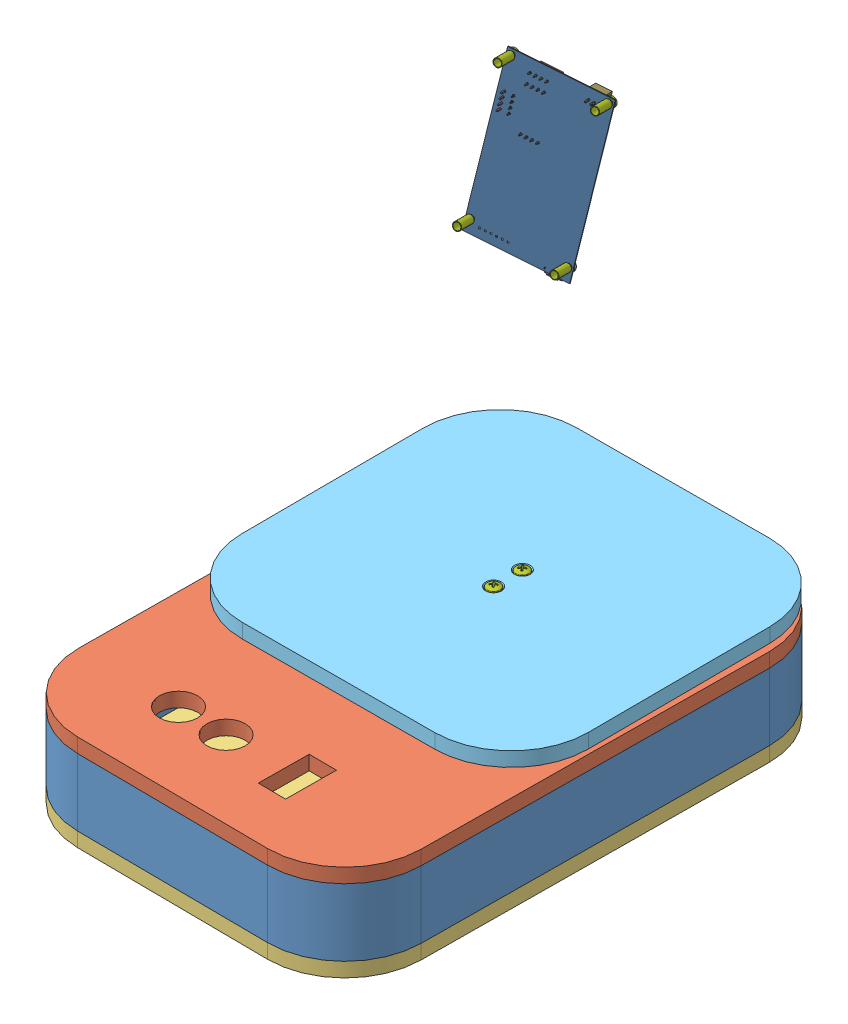
SolidWorks assembly Mainv1, configuration Default. Lengths in mm.
Overall size (261.27 140.54 358.53).
175 component instances, 43 part files, 26 mates.
Components (placement in the parent):
- mail wall-1: mail wall [Default] at (468.1099 74.0645 -181.95) x (-0.999962 0 -0.008727) z (0.008727 0 -0.999962) size (180 35 260)
- top lid-1: top lid [Default] at (468.1099 116.5645 -181.95) x (-0.999962 0 -0.008727) z (0.008727 0 -0.999962) size (180 7.5 260)
- bottom lid-2: bottom lid [Default] at (468.1099 31.5645 -181.95) x (0.999962 0 0.008727) z (-0.008727 0 0.999962) size (180 7.5 260)
- Loadcell-1kg-No Name.step-1: Loadcell-1kg-No Name.step [Default] at (468.4825 94.8439 -197.5959) x (0 0 1) z (-1 0 0) size (91.8 14.23 13.91)
- tray-1: tray [Default] at (468.6751 134.9439 -266.3463) x (0.999991 0 -0.00428) z (0.00428 0 0.999991) size (180 7.5 175)
- Part5-1: Part5 [Default] at origin size (12.6 12.5 27.5)
- pan cross head_am-1: pan cross head_am [B18.6.7M - M3.5 x 0.6 x 35 Type I Cross Recessed PHMS --35N] at (468.4825 128.4614 -232.8459) x (0 -1 0) z (-0.788636 0 0.61486) size (37.57 7 7)
- pan cross head_am-3: pan cross head_am [B18.6.7M - M3.5 x 0.6 x 35 Type I Cross Recessed PHMS --35N] at (468.4825 128.5554 -217.8459) x (0 -1 0) z (0.792721 0 -0.609585) size (37.57 7 7)
- Part1-1: Part1 [Default] at origin size (50 22.7 32.99)
- hex bolt_am-1: hex bolt_am [B18.2.3.5M - Hex bolt M5 x 0.8 x 35 --16N] at (468.8184 72.2139 -162.6607) x (0 1 0) z (0 0 1) size (38.58 9.24 8)
- hex bolt_am-2: hex bolt_am [B18.2.3.5M - Hex bolt M5 x 0.8 x 35 --16N] at (468.8184 72.2139 -177.7301) x (0 1 0) z (0 0 1) size (38.58 9.24 8)
- pcb.step-1: pcb.step [Default] at (347.6655 123.4151 -378.6091) x (-0.974446 0.114203 0.193422) z (-0.214397 -0.216049 -0.952553) size (48.01 79.98 16.61)
  - Board.step-1: Board.step [Default] at origin size (48.01 78.74 0.41)
    - Open CASCADE STEP translator 7.5 2.1.1.step-1: Open CASCADE STEP translator 7.5 2.1.1.step [Default] at (0 0 -0.4115) size (48.01 78.74 0.41)
  - HX711 out.step-1: HX711 out.step [Default] at origin size (10.16 2.54 10.59)
    - Header_4.step-1: Header_4.step [Default] at (27.685 46.598 -0.0051) x (0 -1 0) z (-1 0 0) size (2.54 10.59 10.16)
      - header.step-1: header.step [Default] at origin size (2.54 10.59 2.54)
        - header-0.step-1: header-0.step [Default] at origin size (2.54 8.5 2.54)
        - pin.step-1: pin.step [Default] at (-1.4 0 0) size (0.4 10 1.99)
      - header.step-2: header.step [Default] at (0 0 -2.54) size (2.54 10.59 2.54)
        - header-0.step-1: header-0.step [Default] at origin size (2.54 8.5 2.54)
        - pin.step-1: pin.step [Default] at (-1.4 0 0) size (0.4 10 1.99)
      - header.step-3: header.step [Default] at (0 0 -5.08) size (2.54 10.59 2.54)
        - header-0.step-1: header-0.step [Default] at origin size (2.54 8.5 2.54)
        - pin.step-1: pin.step [Default] at (-1.4 0 0) size (0.4 10 1.99)
      - header.step-4: header.step [Default] at (0 0 -7.62) size (2.54 10.59 2.54)
        - header-0.step-1: header-0.step [Default] at origin size (2.54 8.5 2.54)
        - pin.step-1: pin.step [Default] at (-1.4 0 0) size (0.4 10 1.99)
  - HX711_lc.step-1: HX711_lc.step [Default] at origin size (10.16 2.54 10.59)
    - Header_4.step-1: Header_4.step [Default] at (30.23 66.915 -0.0051) x (0 -1 0) z (-1 0 0) size (2.54 10.59 10.16)
      - header.step-1: header.step [Default] at origin size (2.54 10.59 2.54)
        - header-0.step-1: header-0.step [Default] at origin size (2.54 8.5 2.54)
        - pin.step-1: pin.step [Default] at (-1.4 0 0) size (0.4 10 1.99)
      - header.step-2: header.step [Default] at (0 0 -2.54) size (2.54 10.59 2.54)
        - header-0.step-1: header-0.step [Default] at origin size (2.54 8.5 2.54)
        - pin.step-1: pin.step [Default] at (-1.4 0 0) size (0.4 10 1.99)
      - header.step-3: header.step [Default] at (0 0 -5.08) size (2.54 10.59 2.54)
        - header-0.step-1: header-0.step [Default] at origin size (2.54 8.5 2.54)
        - pin.step-1: pin.step [Default] at (-1.4 0 0) size (0.4 10 1.99)
      - header.step-4: header.step [Default] at (0 0 -7.62) size (2.54 10.59 2.54)
        - header-0.step-1: header-0.step [Default] at origin size (2.54 8.5 2.54)
        - pin.step-1: pin.step [Default] at (-1.4 0 0) size (0.4 10 1.99)
  - usb 2.0.step-1: usb 2.0.step [Default] at origin size (7.8 5.5 3.71)
    - USB3090-30-A--3DModel-STEP-56544.step-1: USB3090-30-A--3DModel-STEP-56544.step [Default] at (7.762 1.514 0) x (1 0 0) z (0 -1 0) size (7.8 3.71 5.5)
  - R 470.step-1: R 470.step [Default] at origin size (2 1.25 0.6)
    - 6201218720.step-1: 6201218720.step [Default] at (15.687 7.62 0) x (1 0 0) z (0 0 1) size (2 1.25 0.6)
      - term1.step-1: term1.step [Default] at (-1 -0.625 0) size (0.35 1.25 0.6)
      - term2.step-1: term2.step [Default] at (0.65 -0.625 0) size (0.35 1.25 0.6)
      - body.step-1: body.step [Default] at (-0.65 -0.6125 0.006) size (1.3 1.22 0.59)
  - R 47k.step-1: R 47k.step [Default] at origin size (2 1.25 0.6)
    - 6062674512.step-1: 6062674512.step [Default] at (18.862 49.53 0) x (-1 0 0) z (0 0 1) size (2 1.25 0.6)
      - term1-1.step-1: term1-1.step [Default] at (-1 -0.625 0) size (0.35 1.25 0.6)
      - term2-2.step-1: term2-2.step [Default] at (0.65 -0.625 0) size (0.35 1.25 0.6)
      - body-3.step-1: body-3.step [Default] at (-0.65 -0.6125 0.006) size (1.3 1.22 0.59)
  - R 15k.step-1: R 15k.step [Default] at origin size (2 1.25 0.6)
    - 7267289360.step-1: 7267289360.step [Default] at (18.937 59.563 0) x (-1 0 0) z (0 0 1) size (2 1.25 0.6)
      - solidBody.step-1: solidBody.step [Default] at origin size (1.95 1.25 0.55)
      - Terminal.step-1: Terminal.step [Default] at origin size (2 1.25 0.6)
      - solidTop.step-1: solidTop.step [Default] at origin size (1.2 1.25 0.02)
  - R5-10K.step-1: R5-10K.step [Default] at origin size (1.6 0.8 0.55)
    - CRG0603F10K_10.step-1: CRG0603F10K_10.step [Default] at (45.212 17.526 0) x (1 0 0) z (0 -1 0) size (1.6 0.55 0.8)
  - R4-10K.step-1: R4-10K.step [Default] at origin size (1.6 0.8 0.55)
    - CRG0603F10K_10.step-1: CRG0603F10K_10.step [Default] at (45.212 22.7965 0) x (-1 0 0) z (0 1 0) size (1.6 0.55 0.8)
  - R3-10K.step-1: R3-10K.step [Default] at origin size (1.6 0.8 0.55)
    - CRG0603F10K_10.step-1: CRG0603F10K_10.step [Default] at (45.212 28.067 0) x (1 0 0) z (0 -1 0) size (1.6 0.55 0.8)
  - R 2k.step-1: R 2k.step [Default] at origin size (2 1.25 0.6)
    - 6062674512.step-1: 6062674512.step [Default] at (15.814 12.319 0) x (-1 0 0) z (0 0 1) size (2 1.25 0.6)
      - term1-1.step-1: term1-1.step [Default] at (-1 -0.625 0) size (0.35 1.25 0.6)
      - term2-2.step-1: term2-2.step [Default] at (0.65 -0.625 0) size (0.35 1.25 0.6)
      - body-3.step-1: body-3.step [Default] at (-0.65 -0.6125 0.006) size (1.3 1.22 0.59)
  - R2-10K.step-1: R2-10K.step [Default] at origin size (1.6 0.8 0.55)
    - CRG0603F10K_10.step-1: CRG0603F10K_10.step [Default] at (22.733 36.195 0) x (-1 0 0) z (0 1 0) size (1.6 0.55 0.8)
  - R1-10K.step-1: R1-10K.step [Default] at origin size (1.6 0.8 0.55)
    - CRG0603F10K_10.step-1: CRG0603F10K_10.step [Default] at (22.733 42.545 0) x (-1 0 0) z (0 1 0) size (1.6 0.55 0.8)
  - MCP73831.step-1: MCP73831.step [Default] at origin size (2.7 2.9 1.45)
    - MCP73831T-5ACI_OT.step-1: MCP73831T-5ACI_OT.step [Default] at (8.255 12.012 0) x (0 -1 0) z (-1 0 0) size (2.9 1.45 2.7)
  - LED.step-1: LED.step [Default] at origin size (3 1 2)
    - KPA-3010CGCK-Base.step-1: KPA-3010CGCK-Base.step [Default] at (16.51 1.651 0.508) x (-1 0 0) z (0 0 -1) size (2.16 1 1.02)
    - KPA-3010CGCK-Base-4.step-1: KPA-3010CGCK-Base-4.step [Default] at (16.51 1.651 0.508) x (-1 0 0) z (0 0 -1) size (3 1 1.22)
    - KPA-3010CGCK-Base-5.step-1: KPA-3010CGCK-Base-5.step [Default] at (16.51 1.651 0.508) x (-1 0 0) z (0 0 -1) size (0.9 1 0)
    - KPA-3010CGCK-Base-6.step-1: KPA-3010CGCK-Base-6.step [Default] at (16.51 1.651 0.508) x (-1 0 0) z (0 0 -1) size (0.8 1 0.02)
    - KPA-3010CGCK-Base-7.step-1: KPA-3010CGCK-Base-7.step [Default] at (16.51 1.651 0.508) x (-1 0 0) z (0 0 -1) size (2.96 1 0.96)
  - battery.step-1: battery.step [Default] at origin size (7.4 5.75 10.4)
    - 6062675712.step-1: 6062675712.step [Default] at (9.274 74.295 0) x (1 0 0) z (0 -1 0) size (7.4 10.4 5.75)
  - load cell.step-1: load cell.step [Default] at origin size (10.16 2.54 10.59)
    - Header_4.step-1: Header_4.step [Default] at (30.099 71.755 -0.0051) x (0 -1 0) z (-1 0 0) size (2.54 10.59 10.16)
      - header.step-1: header.step [Default] at origin size (2.54 10.59 2.54)
        - header-0.step-1: header-0.step [Default] at origin size (2.54 8.5 2.54)
        - pin.step-1: pin.step [Default] at (-1.4 0 0) size (0.4 10 1.99)
      - header.step-2: header.step [Default] at (0 0 -2.54) size (2.54 10.59 2.54)
        - header-0.step-1: header-0.step [Default] at origin size (2.54 8.5 2.54)
        - pin.step-1: pin.step [Default] at (-1.4 0 0) size (0.4 10 1.99)
      - header.step-3: header.step [Default] at (0 0 -5.08) size (2.54 10.59 2.54)
        - header-0.step-1: header-0.step [Default] at origin size (2.54 8.5 2.54)
        - pin.step-1: pin.step [Default] at (-1.4 0 0) size (0.4 10 1.99)
      - header.step-4: header.step [Default] at (0 0 -7.62) size (2.54 10.59 2.54)
        - header-0.step-1: header-0.step [Default] at origin size (2.54 8.5 2.54)
        - pin.step-1: pin.step [Default] at (-1.4 0 0) size (0.4 10 1.99)
  - buttons.step-1: buttons.step [Default] at origin size (2.54 10.16 10.59)
    - Header_4.step-1: Header_4.step [Default] at (39.497 59.817 -0.0051) x (-1 0 0) z (0 1 0) size (2.54 10.59 10.16)
      - header.step-1: header.step [Default] at origin size (2.54 10.59 2.54)
        - header-0.step-1: header-0.step [Default] at origin size (2.54 8.5 2.54)
        - pin.step-1: pin.step [Default] at (-1.4 0 0) size (0.4 10 1.99)
      - header.step-2: header.step [Default] at (0 0 -2.54) size (2.54 10.59 2.54)
        - header-0.step-1: header-0.step [Default] at origin size (2.54 8.5 2.54)
        - pin.step-1: pin.step [Default] at (-1.4 0 0) size (0.4 10 1.99)
      - header.step-3: header.step [Default] at (0 0 -5.08) size (2.54 10.59 2.54)
        - header-0.step-1: header-0.step [Default] at origin size (2.54 8.5 2.54)
        - pin.step-1: pin.step [Default] at (-1.4 0 0) size (0.4 10 1.99)
      - header.step-4: header.step [Default] at (0 0 -7.62) size (2.54 10.59 2.54)
        - header-0.step-1: header-0.step [Default] at origin size (2.54 8.5 2.54)
        - pin.step-1: pin.step [Default] at (-1.4 0 0) size (0.4 10 1.99)
  - OLED.step-1: OLED.step [Default] at origin size (2.54 10.16 16)
    - MTSW-104-22-S-S-420.step-1: MTSW-104-22-S-S-420.step [Default] at (44.831 57.277 0) x (0 -1 0) z (-1 0 0) size (10.16 16 2.54)
      - MTSW-104-22-S-420.step-1: MTSW-104-22-S-420.step [Default] at (0 -2.794 0) size (8.51 16 0.89)
      - MTSW-104-22-S-S-420_body.step-1: MTSW-104-22-S-S-420_body.step [Default] at origin size (10.16 2.54 2.54)
  - ESP-12F.step-1: ESP-12F.step [Default] at origin size (17.7 24.9 3.1)
    - ESP-12F-8.step-1: ESP-12F-8.step [Default] at (33.909 28.956 0) x (1 0 0) z (0 -1 0) size (17.7 3.1 24.9)
  - C5-4.7uF.step-1: C5-4.7uF.step [Default] at origin size (2 1.25 1.45)
    - 885012107013.step-1: 885012107013.step [Default] at (10.345 18.923 0) x (-1 0 0) z (0 0 1) size (2 1.25 1.45)
      - Fillet1.step-1: Fillet1.step [Default] at origin size (0.5 1.25 1.45)
      - Fillet2.step-1: Fillet2.step [Default] at origin size (0.5 1.25 1.45)
      - body2.step-1: body2.step [Default] at origin size (1 1.22 1.42)
  - C4-4.7uF.step-1: C4-4.7uF.step [Default] at origin size (2 1.25 1.45)
    - 885012107013.step-1: 885012107013.step [Default] at (11.245 26.543 0) x (1 0 0) z (0 0 1) size (2 1.25 1.45)
      - Fillet1.step-1: Fillet1.step [Default] at origin size (0.5 1.25 1.45)
      - Fillet2.step-1: Fillet2.step [Default] at origin size (0.5 1.25 1.45)
      - body2.step-1: body2.step [Default] at origin size (1 1.22 1.42)
  - C3-10uF.step-1: C3-10uF.step [Default] at origin size (5.3 4.5 5.5)
    - 865080340001.step-1: 865080340001.step [Default] at (10.737 64.643 0) x (-1 0 0) z (0 0 1) size (5.3 4.5 5.5)
      - Base.step-1: Base.step [Default] at origin size (4.5 4.5 1.6)
      - Pin1Fillet.step-1: Pin1Fillet.step [Default] at origin size (2.25 0.75 0.3)
      - Pin2Fillet.step-1: Pin2Fillet.step [Default] at origin size (2.25 0.75 0.3)
      - Fillet.step-1: Fillet.step [Default] at origin size (4.2 4.2 4.4)
    - 865080340001.step-2: 865080340001.step [Default] at (10.737 64.643 0) x (-1 0 0) z (0 0 1) size (5.3 4.5 5.5)
      - Base.step-1: Base.step [Default] at origin size (4.5 4.5 1.6)
      - Pin1Fillet.step-1: Pin1Fillet.step [Default] at origin size (2.25 0.75 0.3)
      - Pin2Fillet.step-1: Pin2Fillet.step [Default] at origin size (2.25 0.75 0.3)
      - Fillet.step-1: Fillet.step [Default] at origin size (4.2 4.2 4.4)
  - C2-10uF.step-1: C2-10uF.step [Default] at origin size (5.3 4.5 5.5)
    - 865080340001.step-1: 865080340001.step [Default] at (10.737 44.069 0) x (-1 0 0) z (0 0 1) size (5.3 4.5 5.5)
      - Base.step-1: Base.step [Default] at origin size (4.5 4.5 1.6)
      - Pin1Fillet.step-1: Pin1Fillet.step [Default] at origin size (2.25 0.75 0.3)
      - Pin2Fillet.step-1: Pin2Fillet.step [Default] at origin size (2.25 0.75 0.3)
      - Fillet.step-1: Fillet.step [Default] at origin size (4.2 4.2 4.4)
    - 865080340001.step-2: 865080340001.step [Default] at (10.737 44.069 0) x (-1 0 0) z (0 0 1) size (5.3 4.5 5.5)
      - Base.step-1: Base.step [Default] at origin size (4.5 4.5 1.6)
      - Pin1Fillet.step-1: Pin1Fillet.step [Default] at origin size (2.25 0.75 0.3)
      - Pin2Fillet.step-1: Pin2Fillet.step [Default] at origin size (2.25 0.75 0.3)
      - Fillet.step-1: Fillet.step [Default] at origin size (4.2 4.2 4.4)
  - C1-10uF.step-1: C1-10uF.step [Default] at origin size (5.3 4.5 5.5)
    - 865080340001.step-1: 865080340001.step [Default] at (33.583 11.303 0) x (-1 0 0) z (0 0 1) size (5.3 4.5 5.5)
      - Base.step-1: Base.step [Default] at origin size (4.5 4.5 1.6)
      - Pin1Fillet.step-1: Pin1Fillet.step [Default] at origin size (2.25 0.75 0.3)
      - Pin2Fillet.step-1: Pin2Fillet.step [Default] at origin size (2.25 0.75 0.3)
      - Fillet.step-1: Fillet.step [Default] at origin size (4.2 4.2 4.4)
    - 865080340001.step-2: 865080340001.step [Default] at (33.583 11.303 0) x (-1 0 0) z (0 0 1) size (5.3 4.5 5.5)
      - Base.step-1: Base.step [Default] at origin size (4.5 4.5 1.6)
      - Pin1Fillet.step-1: Pin1Fillet.step [Default] at origin size (2.25 0.75 0.3)
      - Pin2Fillet.step-1: Pin2Fillet.step [Default] at origin size (2.25 0.75 0.3)
      - Fillet.step-1: Fillet.step [Default] at origin size (4.2 4.2 4.4)
  - TC2117.step-1: TC2117.step [Default] at origin size (7.13 5.32 1.17)
    - TC2117-3.3VDBTR.step-1: TC2117-3.3VDBTR.step [Default] at (10.864 54.356 0) x (-1 0 0) z (0 0 1) size (7 5.32 1.17)
      - body.step-1: body.step [Default] at origin size (1.3 1.22 0.59)
      - PinsArrayL.step-1: PinsArrayL.step [Default] at origin size (1.75 5.32 1.17)
      - FilletPinR.step-1: FilletPinR.step [Default] at origin size (1.75 3 1.17)
    - TC2117-3.3VDBTR.step-2: TC2117-3.3VDBTR.step [Default] at (10.737 54.356 0) x (-1 0 0) z (0 0 1) size (7 5.32 1.17)
      - body.step-1: body.step [Default] at origin size (1.3 1.22 0.59)
      - PinsArrayL.step-1: PinsArrayL.step [Default] at origin size (1.75 5.32 1.17)
      - FilletPinR.step-1: FilletPinR.step [Default] at origin size (1.75 3 1.17)
- Part36-1: Part36 [Default] at origin size (53.08 79 35.65)
- pan cross head_am-4: pan cross head_am [B18.6.7M - M2.5 x 0.45 x 5 Type I Cross Recessed PHMS --5N] at (303.2042 134.2026 -373.2533) x (0.214397 0.216049 0.952553) z (-0.952107 -0.171442 0.253181) size (7.07 5 5)
- pan cross head_am-5: pan cross head_am [B18.6.7M - M2.5 x 0.45 x 5 Type I Cross Recessed PHMS --5N] at (307.9009 202.1811 -389.7286) x (0.214397 0.216049 0.952553) z (-0.586235 0.808507 -0.05143) size (7.07 5 5)
- pan cross head_am-6: pan cross head_am [B18.6.7M - M2.5 x 0.45 x 5 Type I Cross Recessed PHMS --5N] at (350.2335 197.3439 -398.1596) x (0.214397 0.216049 0.952553) z (0.724601 0.618774 -0.303435) size (7.07 5 5)
- pan cross head_am-7: pan cross head_am [B18.6.7M - M2.5 x 0.45 x 5 Type I Cross Recessed PHMS --5N] at (345.5283 129.2423 -381.6544) x (0.214397 0.216049 0.952553) z (-0.921974 0.36675 0.124331) size (7.07 5 5)
Mates (geometry in assembly coordinates):
- Coincident5: coincident anti-aligned: plane of Loadcell-1kg-No Name.step-1 through (468.4825 107.4439 -197.5959) normal (0 1 0); plane of Part5-1 through (0 107.4439 0) normal (0 -1 0)
- Coincident6: coincident anti-aligned: line of Loadcell-1kg-No Name.step-1 through (474.7825 107.4439 -237.5959) axis (-1 0 0); line of Part5-1 through (462.1825 107.4439 -237.5959) axis (1 0 0)
- Coincident8: coincident aligned: line of Loadcell-1kg-No Name.step-1 through (474.7825 107.4439 -157.5959) axis (0 0 -1); line of Part5-1 through (474.7825 107.4439 -210.0959) axis (0 0 -1)
- Concentric12: concentric aligned: cylinder of Part5-1 through (468.4825 127.4439 -232.8459) axis (0 1 0) radius 1.85; cylinder of pan cross head_am-1 through (468.4825 153.8614 -232.8459) axis (0 1 0) radius 1.75
- Coincident9: coincident aligned: cylinder of tray-1 through (468.4825 127.4439 -232.8459) axis (0 1 0) radius 1.85; circle of Part5-1
- Concentric15: concentric aligned: circle of tray-1; cylinder of pan cross head_am-3 through (468.4825 153.9554 -217.8459) axis (0 1 0) radius 1.75
- Concentric17: concentric aligned: cylinder of Part1-1 through (468.8184 72.1439 -162.6607) axis (0 -1 0) radius 2.65; cylinder of hex bolt_am-1 through (468.8184 72.2139 -162.6607) axis (0 -1 0) radius 2.5
- Concentric18: concentric aligned: cylinder of Part1-1 through (468.8184 72.1439 -177.7301) axis (0 -1 0) radius 2.65; cylinder of hex bolt_am-2 through (468.8184 72.2139 -177.7301) axis (0 -1 0) radius 2.5
- Coincident10: coincident anti-aligned: plane of Part1-1 through (471.4684 75.7939 -177.7301) normal (0 -1 0); plane of hex bolt_am-2 through (464.1996 75.7939 -177.7301) normal (0 1 0)
- Coincident11: coincident anti-aligned: plane of Part1-1 through (471.4684 75.7939 -162.6607) normal (0 -1 0); plane of hex bolt_am-1 through (464.1996 75.7939 -162.6607) normal (0 1 0)
- Coincident16: coincident anti-aligned: line of mail wall-1 through (557.3211 109.0645 -91.168) axis (0.008727 0 -0.999962); line of top lid-1 through (558.8919 109.0645 -271.1612) axis (-0.008727 0 0.999962)
- Coincident17: coincident aligned: line of mail wall-1 through (516.9736 109.0645 -51.5186) axis (-0.999962 0 -0.008727); line of top lid-1 through (516.9736 109.0645 -51.5186) axis (-0.999962 0 -0.008727)
- Coincident18: coincident anti-aligned: line of mail wall-1 through (516.9736 74.0645 -51.5186) axis (-0.999962 0 -0.008727); line of bottom lid-2 through (416.9774 74.0645 -52.3913) axis (0.999962 0 0.008727)
- Coincident19: coincident aligned: line of mail wall-1 through (557.3211 74.0645 -91.168) axis (0.008727 0 -0.999962); line of bottom lid-2 through (557.3211 74.0645 -91.168) axis (0.008727 0 -0.999962)
- Concentric19: concentric aligned: circle of pcb.step-1/Board.step-1/Open CASCADE STEP translator 7.5 2.1.1.step-1; cylinder of Part36-1 through (352.9159 200.047 -386.2417) axis (-0.214397 -0.216049 -0.952553) radius 2
- Concentric20: concentric aligned: circle of pcb.step-1/Board.step-1/Open CASCADE STEP translator 7.5 2.1.1.step-1; cylinder of Part36-1 through (310.5833 204.8841 -377.8108) axis (-0.214397 -0.216049 -0.952553) radius 2
- Concentric21: concentric aligned: circle of pcb.step-1/Board.step-1/Open CASCADE STEP translator 7.5 2.1.1.step-1; cylinder of Part36-1 through (348.2107 131.9454 -369.7365) axis (-0.214397 -0.216049 -0.952553) radius 2
- Concentric22: concentric aligned: circle of pcb.step-1/Board.step-1/Open CASCADE STEP translator 7.5 2.1.1.step-1; cylinder of Part36-1 through (305.8866 136.9057 -361.3354) axis (-0.214397 -0.216049 -0.952553) radius 2
- Concentric23: concentric aligned: cylinder of Part36-1 through (303.7427 134.7452 -370.861) axis (-0.214397 -0.216049 -0.952553) radius 1.7; cylinder of pan cross head_am-4 through (297.7585 128.7149 -397.4481) axis (-0.214397 -0.216049 -0.952553) radius 1.25
- Concentric24: concentric aligned: cylinder of Part36-1 through (346.0668 129.7849 -379.262) axis (-0.214397 -0.216049 -0.952553) radius 1.7; cylinder of pan cross head_am-7 through (336.0138 123.9261 -411.3844) axis (-0.214397 -0.216049 -0.952553) radius 1.25
- Concentric25: concentric aligned: cylinder of Part36-1 through (308.4393 202.7237 -387.3363) axis (-0.214397 -0.216049 -0.952553) radius 1.7; cylinder of pan cross head_am-5 through (302.4552 196.6934 -413.9235) axis (-0.214397 -0.216049 -0.952553) radius 1.25
- Concentric27: concentric aligned: cylinder of Part36-1 through (350.772 197.8865 -395.7672) axis (-0.214397 -0.216049 -0.952553) radius 1.7; cylinder of pan cross head_am-6 through (344.7878 191.8563 -422.3544) axis (-0.214397 -0.216049 -0.952553) radius 1.25
- Coincident23: coincident anti-aligned: plane of pcb.step-1/Board.step-1/Open CASCADE STEP translator 7.5 2.1.1.step-1 through (326.9135 164.3326 -383.2189) normal (-0.214397 -0.216049 -0.952553); plane of pan cross head_am-5 through (309.3277 203.319 -388.1032) normal (0.214397 0.216049 0.952553)
- Coincident24: coincident anti-aligned: plane of pcb.step-1/Board.step-1/Open CASCADE STEP translator 7.5 2.1.1.step-1 through (326.9135 164.3326 -383.2189) normal (-0.214397 -0.216049 -0.952553); plane of pan cross head_am-6 through (351.5024 196.8535 -396.1293) normal (0.214397 0.216049 0.952553)
- Coincident25: coincident anti-aligned: plane of pcb.step-1/Board.step-1/Open CASCADE STEP translator 7.5 2.1.1.step-1 through (326.9135 164.3326 -383.2189) normal (-0.214397 -0.216049 -0.952553); plane of pan cross head_am-4 through (303.3819 135.8578 -371.4641) normal (0.214397 0.216049 0.952553)
- Coincident26: coincident anti-aligned: plane of pcb.step-1/Board.step-1/Open CASCADE STEP translator 7.5 2.1.1.step-1 through (326.9135 164.3326 -383.2189) normal (-0.214397 -0.216049 -0.952553); plane of pan cross head_am-7 through (346.3817 130.8271 -380.0013) normal (0.214397 0.216049 0.952553)
